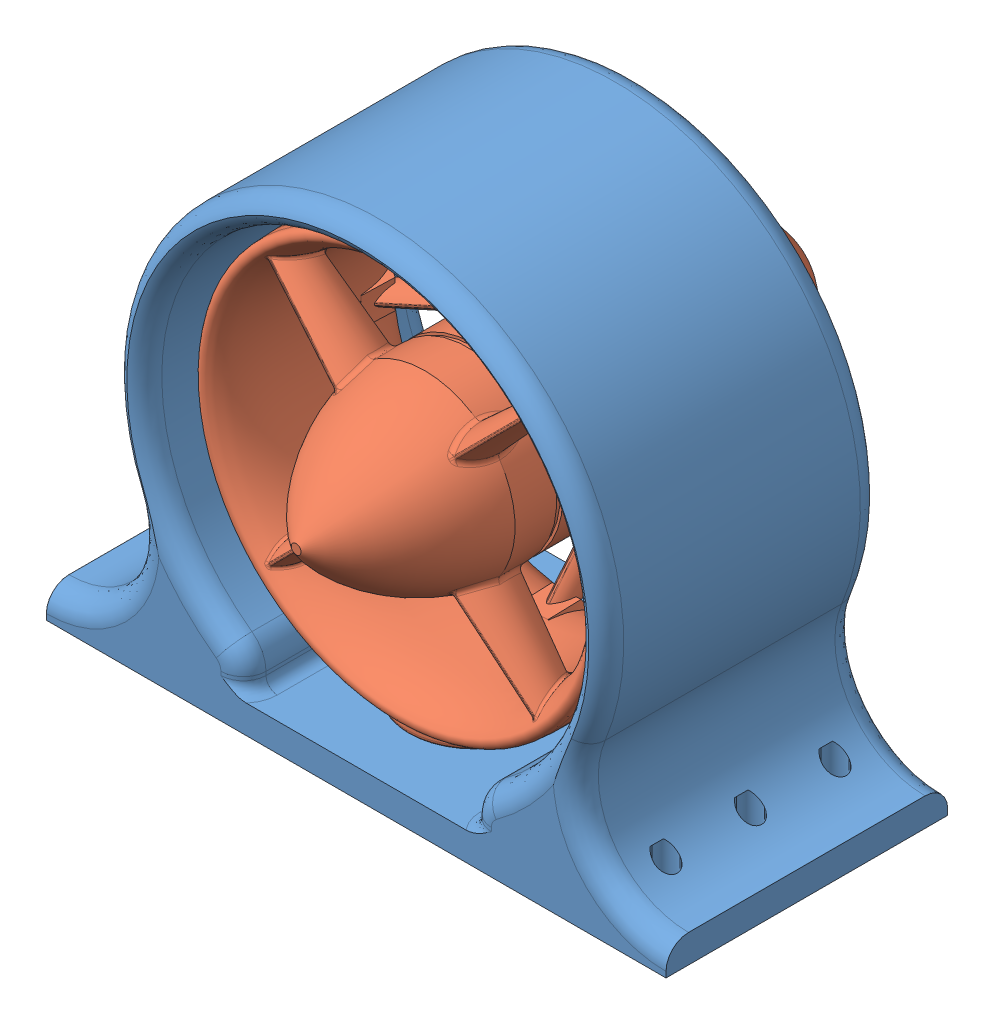
SolidWorks assembly CR-SA-HorizontalThrusterAndMount, configuration Default. Lengths in mm.
Overall size (139.7 110.81 112.68).
2 component instances, 2 part files, 6 mates.
Components (placement in the parent):
- CR-P-0005b-Frame-MotorMount Horizontal-1: CR-P-0005b-Frame-MotorMount Horizontal [Default] at (0 55.5625 -5.427) x (0 -1 0) z (0 0 1) size (110.81 139.7 64.82)
- CR-P-0003-T200-THRUSTER-R1-1: CR-P-0003-T200-THRUSTER-R1 [Default] at (0 55.5625 26.323) x (1 0 0) z (0 0 -1) size (96.71 97.53 112.68)
Mates (geometry in assembly coordinates):
- Coincident1: coincident anti-aligned: plane of CR-P-0005b-Frame-MotorMount Horizontal-1 through (0 0 58.073) normal (0 -1 0)
- Coincident2: coincident aligned: plane of CR-P-0005b-Frame-MotorMount Horizontal-1 through (0 55.5625 -5.427) normal (1 0 0)
- Concentric1: concentric anti-aligned: cylinder of CR-P-0005b-Frame-MotorMount Horizontal-1 through (0 55.5625 58.073) axis (0 0 -1) radius 48.895; circle of CR-P-0003-T200-THRUSTER-R1-1
- Parallel1: parallel anti-aligned: plane of CR-P-0005b-Frame-MotorMount Horizontal-1 through (0 6.35 58.073) normal (0 1 0); plane of CR-P-0003-T200-THRUSTER-R1-1 through (0 6.5625 31.5748) normal (0 -1 0)
- Coincident4: coincident aligned: plane of CR-P-0005b-Frame-MotorMount Horizontal-1 through (0 55.5625 -5.427) normal (1 0 0); plane of CR-P-0003-T200-THRUSTER-R1-1 through (0 55.5625 26.323) normal (1 0 0)
- Distance1: distance = 31.75 mm anti-aligned: plane of CR-P-0005b-Frame-MotorMount Horizontal-1 through (0 55.5625 -5.427) normal (0 0 1); plane of CR-P-0003-T200-THRUSTER-R1-1 through (0 55.5625 26.323) normal (0 0 -1)
